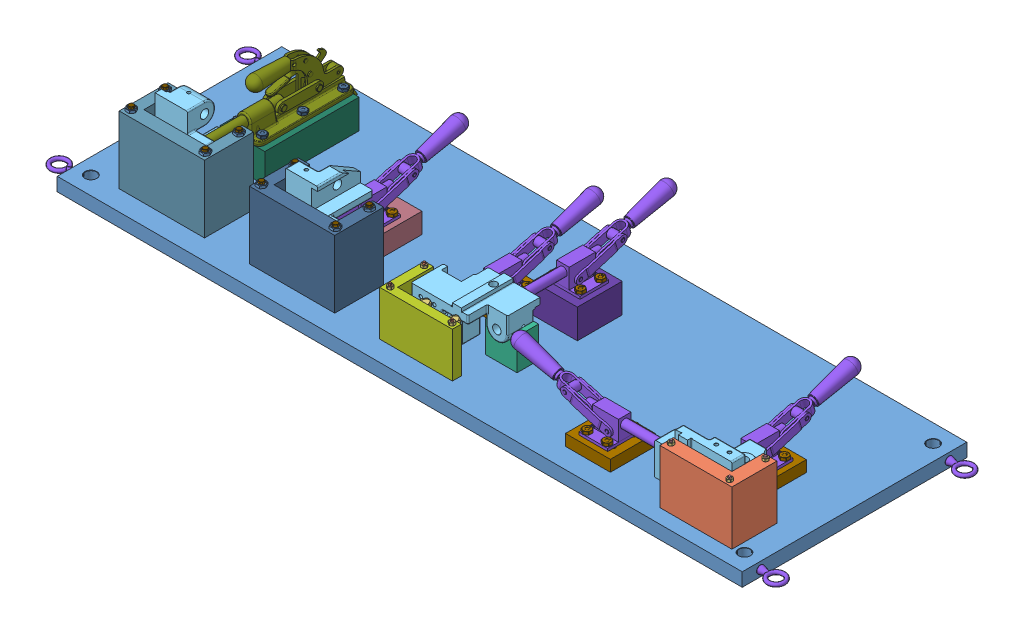
SolidWorks assembly Fixture Assy, configuration Default. Lengths in mm. (continued)
Mates (geometry in assembly coordinates): (continued)
- Coincident182: coincident anti-aligned: plane of Operation 1 Clamp Base-7 through (886.2945 606.2285 944.288) normal (0 1 0); plane of 5222N4_Heavy Duty Reverse-Action Push Toggle Clamp-7 through (854.2945 606.2285 982.288) normal (0 -1 0)
- Coincident183: coincident anti-aligned: plane of Roller Rest Bracket-1 through (1003.0152 704.2285 962.288) normal (-1 0 0); plane of 5222N4_Heavy Duty Reverse-Action Push Toggle Clamp-7 through (1003.0152 641.2285 944.288) normal (1 0 0)
- Distance93: distance = 45 mm aligned: plane of Operation 1 Clamp Base-7 through (836.2945 606.2285 994.288) normal (0 0 1); plane of Base-1 through (-724.9848 581.2285 1039.288) normal (0 0 1)
- Distance94: distance = 45 mm aligned: plane of Opeartion 3 BLock-1 through (322.5123 731.2285 994.288) normal (0 0 1); plane of Base-1 through (-724.9848 581.2285 1039.288) normal (0 0 1)
- Distance95: distance = 88 mm aligned: plane of U - BLock-Operation 2-1 through (422.5123 581.2285 994.288) normal (0 0 1); plane of Vee Block-1 through (570.5123 651.2285 906.288) normal (0 0 1)
- Coincident194: coincident aligned: plane of U - BLock-Operation 2-1 through (422.5123 581.2285 994.288) normal (0 0 1); plane of Opeartion 3 BLock-1 through (322.5123 731.2285 994.288) normal (0 0 1)
- Distance97: distance = 72 mm: cylinder of 2336A124_Locating Pin-18 through (424.5123 662.9738 902.288) axis (-1 0 0) radius 6; plane of U - BLock-Operation 2-1 through (644.5123 581.2285 974.288) normal (0 0 -1)
- Distance98: distance = 10 mm aligned: plane of 2336A124_Locating Pin-18 through (457.5123 671.2285 907.9324) normal (0 1 0); plane of U - BLock-Operation 2-1 through (543.5123 681.2285 974.288) normal (0 1 0)
- Width17: width anti-aligned: plane of Operation 2 Clamp Base-8 through (646.0152 646.2285 677.5673) normal (1 0 0); plane of 5222N4_Heavy Duty Reverse-Action Push Toggle Clamp-8 through (546.0152 646.2285 677.5673) normal (-1 0 0); plane of Operation 2 Clamp Base-8 through (558.0152 652.2285 759.5673) normal (-1 0 0); plane of 5222N4_Heavy Duty Reverse-Action Push Toggle Clamp-8 through (634.0152 652.2285 759.5673) normal (1 0 0)
- Width18: width anti-aligned: plane of Operation 2 Clamp Base-8 through (546.0152 646.2285 677.5673) normal (0 0 -1); plane of 5222N4_Heavy Duty Reverse-Action Push Toggle Clamp-8 through (546.0152 646.2285 777.5673) normal (0 0 1); plane of Operation 2 Clamp Base-8 through (634.0152 652.2285 759.5673) normal (0 0 1); plane of 5222N4_Heavy Duty Reverse-Action Push Toggle Clamp-8 through (634.0152 652.2285 695.5673) normal (0 0 -1)
- Coincident188: coincident anti-aligned: plane of 5222N4_Heavy Duty Reverse-Action Push Toggle Clamp-8 through (558.0152 646.2285 695.5673) normal (0 -1 0); plane of Operation 2 Clamp Base-8 through (596.0152 646.2285 727.5673) normal (0 1 0)
- Coincident193: coincident anti-aligned: plane of Base-1 through (275.0152 581.2285 789.288) normal (0 1 0); plane of Operation 2 Clamp Base-8 through (596.0152 581.2285 727.5673) normal (0 -1 0)
- Coincident195: coincident anti-aligned: plane of Roller Rest Bracket-2 through (457.5123 690.2285 844.288) normal (0 0 -1); plane of 5222N4_Heavy Duty Reverse-Action Push Toggle Clamp-8 through (596.0152 681.2285 844.288) normal (0 0 1)
- Distance100: distance = 6 mm anti-aligned: plane of Operation 1 Clamp Base-4 through (540.0152 606.2285 734.5673) normal (1 0 0); plane of Operation 2 Clamp Base-8 through (546.0152 646.2285 677.5673) normal (-1 0 0)
- Coincident198: coincident anti-aligned: plane of Base-1 through (275.0152 551.2285 789.288) normal (0 -1 0); plane of 93516A178_Bronze Hex Head Screw-2 through (321.0108 551.2285 904.813) normal (0 1 0)
- Coincident199: coincident anti-aligned: plane of Base-1 through (275.0152 551.2285 789.288) normal (0 -1 0); plane of 93516A178_Bronze Hex Head Screw-2 through (321.0108 551.2285 904.813) normal (0 1 0)
- Coincident200: coincident anti-aligned: plane of Base-1 through (275.0152 551.2285 789.288) normal (0 -1 0); plane of 93516A178_Bronze Hex Head Screw-3 through (-139.4885 551.2285 989.288) normal (0 1 0)
- Coincident201: coincident anti-aligned: plane of Base-1 through (275.0152 551.2285 789.288) normal (0 -1 0); plane of 93516A178_Bronze Hex Head Screw-4 through (150.5115 551.2285 914.338) normal (0 1 0)
- Coincident202: coincident anti-aligned: plane of Base-1 through (275.0152 551.2285 789.288) normal (0 -1 0); plane of 93516A178_Bronze Hex Head Screw-5 through (315.5115 551.2285 989.288) normal (0 1 0)
- Coincident203: coincident anti-aligned: plane of Base-1 through (275.0152 551.2285 789.288) normal (0 -1 0); plane of 93516A178_Bronze Hex Head Screw-8 through (31.0108 551.2285 904.813) normal (0 1 0)
- Coincident204: coincident anti-aligned: plane of Base-1 through (275.0152 551.2285 789.288) normal (0 -1 0); plane of 93516A178_Bronze Hex Head Screw-9 through (-133.9892 551.2285 904.813) normal (0 1 0)
- Coincident205: coincident anti-aligned: plane of Base-1 through (275.0152 551.2285 789.288) normal (0 -1 0); plane of 93516A178_Bronze Hex Head Screw-7 through (150.5115 551.2285 989.288) normal (0 1 0)
- Coincident206: coincident anti-aligned: plane of Base-1 through (275.0152 551.2285 789.288) normal (0 -1 0); plane of 93516A178_Bronze Hex Head Screw-6 through (31.0108 551.2285 979.763) normal (0 1 0)
- Distance101: distance = 10 mm aligned: plane of Opeartion 3 BLock-1 through (297.5123 731.2285 885.288) normal (0 0 -1); plane of 93516A178_Bronze Hex Head Screw-2 through (304.513 543.291 895.288) normal (0 0 -1)
- Width19: width: plane of Opeartion 3 BLock-1 through (322.5123 731.2285 885.288) normal (1 0 0); plane of Opeartion 3 BLock-1 through (297.5123 731.2285 964.288) normal (-1 0 0); cylinder of 93516A178_Bronze Hex Head Screw-2 through (310.0123 741.7285 904.813) axis (0 1 0) radius 6.35
- Width20: width: plane of Opeartion 3 BLock-1 through (132.5123 731.2285 994.288) normal (-1 0 0); plane of Opeartion 3 BLock-1 through (157.5123 731.2285 885.288) normal (1 0 0); cylinder of 93516A178_Bronze Hex Head Screw-4 through (145.0123 741.7285 904.813) axis (0 1 0) radius 6.35
- Width21: width: plane of Opeartion 3 BLock-1 through (157.5123 731.2285 885.288) normal (1 0 0); plane of Opeartion 3 BLock-1 through (132.5123 731.2285 994.288) normal (-1 0 0); cylinder of 93516A178_Bronze Hex Head Screw-7 through (145.0123 741.7285 979.763) axis (0 1 0) radius 6.35
- Width22: width: plane of Opeartion 3 BLock-1 through (297.5123 731.2285 964.288) normal (-1 0 0); plane of Opeartion 3 BLock-1 through (322.5123 731.2285 885.288) normal (1 0 0); cylinder of 93516A178_Bronze Hex Head Screw-5 through (310.0123 741.7285 979.763) axis (0 1 0) radius 6.35
- Width23: width: plane of Opeartion 4 BLock-2 through (32.5123 731.2285 885.288) normal (1 0 0); plane of Opeartion 4 BLock-2 through (7.5123 731.2285 964.288) normal (-1 0 0); cylinder of 93516A178_Bronze Hex Head Screw-8 through (20.0123 741.7285 904.813) axis (0 1 0) radius 6.35
- Width24: width: plane of Opeartion 4 BLock-2 through (7.5123 731.2285 964.288) normal (-1 0 0); plane of Opeartion 4 BLock-2 through (32.5123 731.2285 885.288) normal (1 0 0); cylinder of 93516A178_Bronze Hex Head Screw-6 through (20.0123 741.7285 979.763) axis (0 1 0) radius 6.35
- Width25: width: plane of Opeartion 4 BLock-2 through (-132.4877 731.2285 885.288) normal (1 0 0); plane of Opeartion 4 BLock-2 through (-157.4877 731.2285 994.288) normal (-1 0 0); cylinder of 93516A178_Bronze Hex Head Screw-9 through (-144.9877 741.7285 904.813) axis (0 1 0) radius 6.35
- Width26: width: plane of Opeartion 4 BLock-2 through (-157.4877 731.2285 994.288) normal (-1 0 0); plane of Opeartion 4 BLock-2 through (-132.4877 731.2285 885.288) normal (1 0 0); cylinder of 93516A178_Bronze Hex Head Screw-3 through (-144.9877 741.7285 979.763) axis (0 1 0) radius 6.35
- Coincident210: coincident aligned: plane of 93516A178_Bronze Hex Head Screw-2 through (304.513 543.291 895.288) normal (0 0 -1); plane of 93516A178_Bronze Hex Head Screw-4 through (139.513 543.291 895.288) normal (0 0 -1)
- Coincident211: coincident aligned: plane of 93516A178_Bronze Hex Head Screw-2 through (304.513 543.291 895.288) normal (0 0 -1); plane of 93516A178_Bronze Hex Head Screw-8 through (14.513 543.291 895.288) normal (0 0 -1)
- Coincident212: coincident aligned: plane of 93516A178_Bronze Hex Head Screw-8 through (14.513 543.291 895.288) normal (0 0 -1); plane of 93516A178_Bronze Hex Head Screw-9 through (-150.487 543.291 895.288) normal (0 0 -1)
- Distance102: distance = 5 mm aligned: plane of 93516A178_Bronze Hex Head Screw-5 through (315.5115 543.291 989.288) normal (0 0 1); plane of Opeartion 3 BLock-1 through (322.5123 731.2285 994.288) normal (0 0 1)
- Coincident214: coincident aligned: plane of 93516A178_Bronze Hex Head Screw-5 through (315.5115 543.291 989.288) normal (0 0 1); plane of 93516A178_Bronze Hex Head Screw-7 through (150.5115 543.291 989.288) normal (0 0 1)
- Coincident215: coincident aligned: plane of 93516A178_Bronze Hex Head Screw-6 through (25.5115 543.291 989.288) normal (0 0 1); plane of 93516A178_Bronze Hex Head Screw-7 through (150.5115 543.291 989.288) normal (0 0 1)
- Coincident216: coincident aligned: plane of 93516A178_Bronze Hex Head Screw-3 through (-139.4885 543.291 989.288) normal (0 0 1); plane of 93516A178_Bronze Hex Head Screw-6 through (25.5115 543.291 989.288) normal (0 0 1)
- Coincident220: coincident anti-aligned: plane of Opeartion 3 BLock-1 through (227.5123 731.2285 994.288) normal (0 1 0); plane of 98886A736_High-Strength High-Temperature PEEK Hex Nut-2 through (310.0123 731.2285 904.813) normal (0 -1 0)
- Concentric3: concentric aligned: circle of 93516A178_Bronze Hex Head Screw-2; circle of 98886A736_High-Strength High-Temperature PEEK Hex Nut-2
- Coincident221: coincident anti-aligned: plane of Opeartion 3 BLock-1 through (227.5123 731.2285 994.288) normal (0 1 0); plane of 98886A736_High-Strength High-Temperature PEEK Hex Nut-3 through (310.0123 731.2285 979.763) normal (0 -1 0)
- Concentric4: concentric anti-aligned: circle of 93516A178_Bronze Hex Head Screw-5; circle of 98886A736_High-Strength High-Temperature PEEK Hex Nut-3
- Concentric5: concentric anti-aligned: circle of 93516A178_Bronze Hex Head Screw-7; circle of 98886A736_High-Strength High-Temperature PEEK Hex Nut-4
- Coincident222: coincident anti-aligned: plane of Opeartion 3 BLock-1 through (227.5123 731.2285 994.288) normal (0 1 0); plane of 98886A736_High-Strength High-Temperature PEEK Hex Nut-4 through (145.0123 731.2285 979.763) normal (0 -1 0)
- Coincident223: coincident anti-aligned: plane of Opeartion 3 BLock-1 through (227.5123 731.2285 994.288) normal (0 1 0); plane of 98886A736_High-Strength High-Temperature PEEK Hex Nut-5 through (145.0123 731.2285 904.813) normal (0 -1 0)
- Concentric6: concentric anti-aligned: circle of 93516A178_Bronze Hex Head Screw-4; circle of 98886A736_High-Strength High-Temperature PEEK Hex Nut-5
- Coincident224: coincident anti-aligned: plane of Opeartion 4 BLock-2 through (-62.4877 731.2285 994.288) normal (0 1 0); plane of 98886A736_High-Strength High-Temperature PEEK Hex Nut-9 through (20.0123 731.2285 904.813) normal (0 -1 0)
- Concentric7: concentric anti-aligned: circle of 93516A178_Bronze Hex Head Screw-8; circle of 98886A736_High-Strength High-Temperature PEEK Hex Nut-9
- Coincident225: coincident anti-aligned: plane of Opeartion 4 BLock-2 through (-62.4877 731.2285 994.288) normal (0 1 0); plane of 98886A736_High-Strength High-Temperature PEEK Hex Nut-8 through (20.0123 731.2285 979.763) normal (0 -1 0)
- Concentric8: concentric anti-aligned: circle of 93516A178_Bronze Hex Head Screw-6; circle of 98886A736_High-Strength High-Temperature PEEK Hex Nut-8
- Coincident226: coincident anti-aligned: plane of Opeartion 4 BLock-2 through (-62.4877 731.2285 994.288) normal (0 1 0); plane of 98886A736_High-Strength High-Temperature PEEK Hex Nut-6 through (-144.9877 731.2285 979.763) normal (0 -1 0)
- Concentric9: concentric anti-aligned: circle of 93516A178_Bronze Hex Head Screw-3; circle of 98886A736_High-Strength High-Temperature PEEK Hex Nut-6
- Coincident227: coincident anti-aligned: plane of Opeartion 4 BLock-2 through (-62.4877 731.2285 994.288) normal (0 1 0); plane of 98886A736_High-Strength High-Temperature PEEK Hex Nut-7 through (-144.9877 731.2285 904.813) normal (0 -1 0)
- Concentric10: concentric anti-aligned: circle of 93516A178_Bronze Hex Head Screw-9; circle of 98886A736_High-Strength High-Temperature PEEK Hex Nut-7
- Coincident229: coincident anti-aligned: plane of Base-1 through (275.0152 551.2285 789.288) normal (0 -1 0); plane of 91268A514_High-Strength Grade 8 Steel Hex Head Screw-1 through (435.7202 551.2285 899.288) normal (0 1 0)
- Coincident230: coincident anti-aligned: plane of Base-1 through (275.0152 551.2285 789.288) normal (0 -1 0); plane of 91268A514_High-Strength Grade 8 Steel Hex Head Screw-2 through (438.7694 551.2285 989.288) normal (0 1 0)
- Coincident231: coincident anti-aligned: plane of Base-1 through (275.0152 551.2285 789.288) normal (0 -1 0); plane of 91268A514_High-Strength Grade 8 Steel Hex Head Screw-3 through (573.956 551.2285 990.7038) normal (0 1 0)
- Distance103: distance = 5 mm aligned: plane of 91268A514_High-Strength Grade 8 Steel Hex Head Screw-2 through (438.7694 547.2598 989.288) normal (0 0 1); plane of U - BLock-Operation 2-1 through (422.5123 581.2285 994.288) normal (0 0 1)
- Distance104: distance = 5 mm aligned: plane of 91268A514_High-Strength Grade 8 Steel Hex Head Screw-1 through (429.3044 547.2598 899.288) normal (0 0 -1); plane of U - BLock-Operation 2-1 through (442.5123 581.2285 894.288) normal (0 0 -1)
- Distance105: distance = 5 mm aligned: plane of 91268A514_High-Strength Grade 8 Steel Hex Head Screw-3 through (579.5123 547.2598 981.0801) normal (1 0 0); plane of U - BLock-Operation 2-1 through (584.5123 581.2285 894.288) normal (1 0 0)
- Width32: width: plane of U - BLock-Operation 2-1 through (422.5123 581.2285 994.288) normal (0 0 1); plane of U - BLock-Operation 2-1 through (644.5123 581.2285 974.288) normal (0 0 -1); cylinder of 91268A514_High-Strength Grade 8 Steel Hex Head Screw-3 through (573.956 538.5335 984.288) axis (0 1 0) radius 3.175
- Width34: width: plane of U - BLock-Operation 2-1 through (422.5123 581.2285 894.288) normal (-1 0 0); plane of U - BLock-Operation 2-1 through (442.5123 581.2285 974.288) normal (1 0 0); cylinder of 91268A514_High-Strength Grade 8 Steel Hex Head Screw-1 through (432.5123 538.5335 904.8443) axis (0 1 0) radius 3.175
- Coincident243: coincident anti-aligned: plane of U - BLock-Operation 2-1 through (543.5123 681.2285 974.288) normal (0 1 0); plane of 95462A029_Medium-Strength Steel Hex Nut-1 through (435.5615 681.2285 983.7318) normal (0 -1 0)
- Concentric11: concentric anti-aligned: circle of 91268A514_High-Strength Grade 8 Steel Hex Head Screw-2; circle of 95462A029_Medium-Strength Steel Hex Nut-1
- Coincident244: coincident anti-aligned: plane of U - BLock-Operation 2-1 through (543.5123 681.2285 974.288) normal (0 1 0); plane of 95462A029_Medium-Strength Steel Hex Nut-2 through (432.5123 681.2285 904.8443) normal (0 -1 0)
- Concentric12: concentric aligned: circle of 91268A514_High-Strength Grade 8 Steel Hex Head Screw-1; circle of 95462A029_Medium-Strength Steel Hex Nut-2
- Coincident245: coincident anti-aligned: plane of U - BLock-Operation 2-1 through (543.5123 681.2285 974.288) normal (0 1 0); plane of 95462A029_Medium-Strength Steel Hex Nut-4 through (573.956 681.2285 984.288) normal (0 -1 0)
- Concentric13: concentric anti-aligned: circle of 91268A514_High-Strength Grade 8 Steel Hex Head Screw-3; circle of 95462A029_Medium-Strength Steel Hex Nut-4
- Coincident248: coincident anti-aligned: plane of Base-1 through (275.0152 551.2285 789.288) normal (0 -1 0); plane of 91251A562_Black-Oxide Alloy Steel Socket Head Screw-1 through (1204.5795 551.2285 1000.433) normal (0 1 0)
- Coincident249: coincident anti-aligned: plane of Base-1 through (275.0152 551.2285 789.288) normal (0 -1 0); plane of 91251A562_Black-Oxide Alloy Steel Socket Head Screw-3 through (1069.5123 551.2285 995.463) normal (0 1 0)
- Coincident250: coincident anti-aligned: plane of Base-1 through (275.0152 551.2285 789.288) normal (0 -1 0); plane of 91251A562_Black-Oxide Alloy Steel Socket Head Screw-2 through (1205.0152 551.2285 920.463) normal (0 1 0)
- Width35: width: plane of U_Block-1 through (1220.0152 701.2285 907.288) normal (1 0 0); plane of U_Block-1 through (1190.0152 701.2285 977.288) normal (-1 0 0); cylinder of 91251A562_Black-Oxide Alloy Steel Socket Head Screw-2 through (1205.0152 542.1046 917.288) axis (0 1 0) radius 3.2258
- Width36: width: plane of U_Block-1 through (1190.0152 701.2285 977.288) normal (-1 0 0); plane of U_Block-1 through (1220.0152 701.2285 907.288) normal (1 0 0); cylinder of 91251A562_Black-Oxide Alloy Steel Socket Head Screw-1 through (1205.0152 542.1046 997.288) axis (0 1 0) radius 3.2258
- Width37: width: plane of U_Block-1 through (991.0152 701.2285 977.288) normal (0 0 -1); plane of U_Block-1 through (1220.0152 701.2285 1007.288) normal (0 0 1); cylinder of 91251A562_Black-Oxide Alloy Steel Socket Head Screw-3 through (1069.5123 542.1046 992.288) axis (0 1 0) radius 3.2258
- Distance109: distance = 10 mm: cylinder of 91251A562_Black-Oxide Alloy Steel Socket Head Screw-3 through (1069.5123 542.1046 992.288) axis (0 1 0) radius 3.2258; plane of U_Block-1 through (1059.5123 701.2285 1007.288) normal (-1 0 0)
- Distance110: distance = 10 mm: cylinder of 91251A562_Black-Oxide Alloy Steel Socket Head Screw-1 through (1205.0152 542.1046 997.288) axis (0 1 0) radius 3.2258; plane of U_Block-1 through (1220.0152 701.2285 1007.288) normal (0 0 1)
- Distance111: distance = 10 mm: cylinder of 91251A562_Black-Oxide Alloy Steel Socket Head Screw-2 through (1205.0152 542.1046 917.288) axis (0 1 0) radius 3.2258; plane of U_Block-1 through (1190.0152 701.2285 907.288) normal (0 0 -1)
- Coincident251: coincident anti-aligned: plane of U_Block-1 through (1090.5152 701.2285 977.288) normal (0 1 0); plane of 95462A029_Medium-Strength Steel Hex Nut-5 through (1069.5123 701.2285 992.288) normal (0 -1 0)
- Concentric14: concentric aligned: circle of 91251A562_Black-Oxide Alloy Steel Socket Head Screw-3; circle of 95462A029_Medium-Strength Steel Hex Nut-5
- Coincident252: coincident anti-aligned: plane of U_Block-1 through (1090.5152 701.2285 977.288) normal (0 1 0); plane of 95462A029_Medium-Strength Steel Hex Nut-6 through (1205.0152 701.2285 997.288) normal (0 -1 0)
- Concentric15: concentric anti-aligned: circle of 91251A562_Black-Oxide Alloy Steel Socket Head Screw-1; circle of 95462A029_Medium-Strength Steel Hex Nut-6
- Coincident253: coincident anti-aligned: plane of U_Block-1 through (1090.5152 701.2285 977.288) normal (0 1 0); plane of 95462A029_Medium-Strength Steel Hex Nut-7 through (1205.0152 701.2285 917.288) normal (0 -1 0)
- Concentric16: concentric anti-aligned: circle of 91251A562_Black-Oxide Alloy Steel Socket Head Screw-2; circle of 95462A029_Medium-Strength Steel Hex Nut-7
- Coincident2551: coincident anti-aligned: plane of Base-1 through (275.0152 551.2285 789.288) normal (0 -1 0); plane of 91257A550_Zinc Yellow-Chromate Plated Hex Head Screw (1)-1 through (631.3915 551.2285 693.6798) normal (0 1 0)
- Coincident2561: coincident anti-aligned: plane of Base-1 through (275.0152 551.2285 789.288) normal (0 -1 0); plane of 91257A550_Zinc Yellow-Chromate Plated Hex Head Screw (1)-2 through (554.2231 551.2285 693.6798) normal (0 1 0)
- Coincident2571: coincident anti-aligned: plane of Base-1 through (275.0152 551.2285 789.288) normal (0 -1 0); plane of 91257A550_Zinc Yellow-Chromate Plated Hex Head Screw (1)-3 through (554.2231 551.2285 772.5673) normal (0 1 0)
- Coincident2581: coincident anti-aligned: plane of Base-1 through (275.0152 551.2285 789.288) normal (0 -1 0); plane of 91257A550_Zinc Yellow-Chromate Plated Hex Head Screw (1)-4 through (631.3915 551.2285 772.5673) normal (0 1 0)
- Distance112: distance = 5 mm aligned: plane of Operation 2 Clamp Base-8 through (546.0152 646.2285 677.5673) normal (0 0 -1); plane of 91257A550_Zinc Yellow-Chromate Plated Hex Head Screw (1)-1 through (631.3915 546.8629 682.5673) normal (0 0 -1)
- Distance113: distance = 5 mm aligned: plane of 91257A550_Zinc Yellow-Chromate Plated Hex Head Screw (1)-4 through (637.8073 546.8629 772.5673) normal (0 0 1); plane of Operation 2 Clamp Base-8 through (546.0152 646.2285 777.5673) normal (0 0 1)
- Distance114: distance = 5 mm aligned: plane of 91257A550_Zinc Yellow-Chromate Plated Hex Head Screw (1)-3 through (560.6389 546.8629 772.5673) normal (0 0 1); plane of Operation 2 Clamp Base-8 through (546.0152 646.2285 777.5673) normal (0 0 1)
- Distance115: distance = 5 mm aligned: plane of Operation 2 Clamp Base-8 through (546.0152 646.2285 677.5673) normal (0 0 -1); plane of 91257A550_Zinc Yellow-Chromate Plated Hex Head Screw (1)-2 through (554.2231 546.8629 682.5673) normal (0 0 -1)
- Distance116: distance = 5 mm: line of 91257A550_Zinc Yellow-Chromate Plated Hex Head Screw (1)-1 through (641.0152 547.3592 688.1236) axis (0 1 0); plane of Operation 2 Clamp Base-8 through (646.0152 646.2285 677.5673) normal (1 0 0)
- Parallel4: parallel aligned: line of 91257A550_Zinc Yellow-Chromate Plated Hex Head Screw (1)-1 through (641.0152 547.3592 688.1236) axis (0 1 0); line of 91257A550_Zinc Yellow-Chromate Plated Hex Head Screw (1)-4 through (641.0152 547.3592 767.0111) axis (0 1 0)
- Distance117: distance = 5 mm: point of 91257A550_Zinc Yellow-Chromate Plated Hex Head Screw (1)-2; plane of Operation 2 Clamp Base-8 through (546.0152 646.2285 677.5673) normal (-1 0 0)
- Distance118: distance = 5 mm: line of 91257A550_Zinc Yellow-Chromate Plated Hex Head Screw (1)-3 through (551.0152 547.3592 767.0111) axis (0 1 0); plane of Operation 2 Clamp Base-8 through (546.0152 646.2285 677.5673) normal (-1 0 0)
- Coincident2583: coincident anti-aligned: plane of Base-1 through (275.0152 551.2285 789.288) normal (0 -1 0); plane of 91257A550_Zinc Yellow-Chromate Plated Hex Head Screw (1)-8 through (-10.1927 551.2285 631.6331) normal (0 1 0)
- Coincident2584: coincident anti-aligned: plane of Base-1 through (275.0152 551.2285 789.288) normal (0 -1 0); plane of 91257A550_Zinc Yellow-Chromate Plated Hex Head Screw (1)-6 through (-16.6085 551.2285 820.5206) normal (0 1 0)
- Coincident2585: coincident anti-aligned: plane of Base-1 through (275.0152 551.2285 789.288) normal (0 -1 0); plane of 91257A550_Zinc Yellow-Chromate Plated Hex Head Screw (1)-5 through (-87.3611 551.2285 820.5206) normal (0 1 0)
- Coincident2586: coincident anti-aligned: plane of Base-1 through (275.0152 551.2285 789.288) normal (0 -1 0); plane of 91257A550_Zinc Yellow-Chromate Plated Hex Head Screw (1)-7 through (-93.7769 551.2285 631.6331) normal (0 1 0)
- Distance119: distance = 5 mm aligned: plane of 91257A550_Zinc Yellow-Chromate Plated Hex Head Screw (1)-8 through (-16.6085 546.8629 620.5206) normal (0 0 -1); plane of Op 4 Clamp base-6 through (-101.9848 646.2285 615.5206) normal (0 0 -1)
- Distance120: distance = 5 mm: line of 91257A550_Zinc Yellow-Chromate Plated Hex Head Screw (1)-8 through (-6.9848 547.3592 626.0769) axis (0 1 0); plane of Op 4 Clamp base-6 through (-1.9848 646.2285 615.5206) normal (1 0 0)
- Coincident2589: coincident aligned: plane of 91257A550_Zinc Yellow-Chromate Plated Hex Head Screw (1)-7 through (-93.7769 546.8629 620.5206) normal (0 0 -1); plane of 91257A550_Zinc Yellow-Chromate Plated Hex Head Screw (1)-8 through (-16.6085 546.8629 620.5206) normal (0 0 -1)
- Distance121: distance = 5 mm: line of 91257A550_Zinc Yellow-Chromate Plated Hex Head Screw (1)-7 through (-96.9848 547.3592 626.0769) axis (0 1 0); plane of Op 4 Clamp base-6 through (-101.9848 646.2285 615.5206) normal (-1 0 0)
- Distance122: distance = 5 mm aligned: plane of 91257A550_Zinc Yellow-Chromate Plated Hex Head Screw (1)-6 through (-10.1927 546.8629 820.5206) normal (0 0 1); plane of Op 4 Clamp base-6 through (-101.9848 646.2285 825.5206) normal (0 0 1)
- Distance123: distance = 5 mm aligned: plane of 91257A550_Zinc Yellow-Chromate Plated Hex Head Screw (1)-5 through (-87.3611 546.8629 820.5206) normal (0 0 1); plane of Op 4 Clamp base-6 through (-101.9848 646.2285 825.5206) normal (0 0 1)
- Distance124: distance = 5 mm: line of 91257A550_Zinc Yellow-Chromate Plated Hex Head Screw (1)-6 through (-6.9848 547.3592 814.9644) axis (0 1 0); plane of Op 4 Clamp base-6 through (-1.9848 646.2285 615.5206) normal (1 0 0)
- Distance125: distance = 5 mm: plane of Op 4 Clamp base-6 through (-101.9848 646.2285 615.5206) normal (-1 0 0); line of 91257A550_Zinc Yellow-Chromate Plated Hex Head Screw (1)-5 through (-96.9848 547.3592 814.9644) axis (0 1 0)
- Coincident2595: coincident anti-aligned: plane of Base-1 through (275.0152 551.2285 789.288) normal (0 -1 0); plane of 91257A552_Zinc Yellow-Chromate Plated Hex Head Screw-2 through (253.3915 551.2285 761.6798) normal (0 1 0)
- Coincident2607: coincident anti-aligned: plane of Base-1 through (275.0152 551.2285 789.288) normal (0 -1 0); plane of 91257A552_Zinc Yellow-Chromate Plated Hex Head Screw-4 through (176.2231 551.2285 761.6798) normal (0 1 0)
- Coincident2597: coincident anti-aligned: plane of Base-1 through (275.0152 551.2285 789.288) normal (0 -1 0); plane of 91257A552_Zinc Yellow-Chromate Plated Hex Head Screw-3 through (253.3915 551.2285 840.5673) normal (0 1 0)
- Coincident2598: coincident anti-aligned: plane of Base-1 through (275.0152 551.2285 789.288) normal (0 -1 0); plane of 91257A552_Zinc Yellow-Chromate Plated Hex Head Screw-1 through (176.2231 551.2285 840.5673) normal (0 1 0)
- Distance126: distance = 5 mm aligned: plane of Operation 3 Clamp Base-5 through (168.0152 626.2285 745.5673) normal (0 0 -1); plane of 91257A552_Zinc Yellow-Chromate Plated Hex Head Screw-2 through (253.3915 546.8629 750.5673) normal (0 0 -1)
- Distance127: distance = 5 mm aligned: plane of 91257A552_Zinc Yellow-Chromate Plated Hex Head Screw-4 through (176.2231 546.8629 750.5673) normal (0 0 -1); plane of Operation 3 Clamp Base-5 through (168.0152 626.2285 745.5673) normal (0 0 -1)
- Distance128: distance = 5 mm aligned: plane of 91257A552_Zinc Yellow-Chromate Plated Hex Head Screw-3 through (259.8073 546.8629 840.5673) normal (0 0 1); plane of Operation 3 Clamp Base-5 through (168.0152 626.2285 845.5673) normal (0 0 1)
- Distance129: distance = 5 mm aligned: plane of 91257A552_Zinc Yellow-Chromate Plated Hex Head Screw-1 through (182.6389 546.8629 840.5673) normal (0 0 1); plane of Operation 3 Clamp Base-5 through (168.0152 626.2285 845.5673) normal (0 0 1)
- Distance130: distance = 5 mm: plane of 91257A552_Zinc Yellow-Chromate Plated Hex Head Screw-2; plane of Operation 3 Clamp Base-5 through (268.0152 626.2285 745.5673) normal (1 0 0)
- Distance131: distance = 5 mm: plane of Operation 3 Clamp Base-5 through (268.0152 626.2285 745.5673) normal (1 0 0); line of 91257A552_Zinc Yellow-Chromate Plated Hex Head Screw-3 through (263.0152 547.3592 835.0111) axis (0 1 0)
- Distance132: distance = 5 mm: plane of Operation 3 Clamp Base-5 through (168.0152 626.2285 745.5673) normal (-1 0 0); line of 91257A552_Zinc Yellow-Chromate Plated Hex Head Screw-4 through (173.0152 547.3592 756.1236) axis (0 1 0)
- Distance133: distance = 5 mm: plane of Operation 3 Clamp Base-5 through (168.0152 626.2285 745.5673) normal (-1 0 0); line of 91257A552_Zinc Yellow-Chromate Plated Hex Head Screw-1 through (173.0152 547.3592 835.0111) axis (0 1 0)
- Coincident2608: coincident anti-aligned: plane of Base-1 through (275.0152 551.2285 789.288) normal (0 -1 0); plane of 91257A546_Zinc Yellow-Chromate Plated Hex Head Screw-1 through (525.3915 551.2285 750.6798) normal (0 1 0)
- Coincident2609: coincident anti-aligned: plane of Base-1 through (275.0152 551.2285 789.288) normal (0 -1 0); plane of 91257A546_Zinc Yellow-Chromate Plated Hex Head Screw-4 through (448.2231 551.2285 750.6798) normal (0 1 0)
- Coincident2610: coincident anti-aligned: plane of Base-1 through (275.0152 551.2285 789.288) normal (0 -1 0); plane of 91257A546_Zinc Yellow-Chromate Plated Hex Head Screw-3 through (525.3915 551.2285 829.5673) normal (0 1 0)
- Coincident2611: coincident anti-aligned: plane of Base-1 through (275.0152 551.2285 789.288) normal (0 -1 0); plane of 91257A546_Zinc Yellow-Chromate Plated Hex Head Screw-2 through (448.2231 551.2285 829.5673) normal (0 1 0)
- Coincident2612: coincident anti-aligned: plane of Base-1 through (275.0152 551.2285 789.288) normal (0 -1 0); plane of 91257A546_Zinc Yellow-Chromate Plated Hex Head Screw-5 through (844.5024 551.2285 989.288) normal (0 1 0)
- Coincident2613: coincident anti-aligned: plane of Base-1 through (275.0152 551.2285 789.288) normal (0 -1 0); plane of 91257A546_Zinc Yellow-Chromate Plated Hex Head Screw-6 through (844.5024 551.2285 910.4005) normal (0 1 0)
- Coincident2614: coincident anti-aligned: plane of Base-1 through (275.0152 551.2285 789.288) normal (0 -1 0); plane of 91257A546_Zinc Yellow-Chromate Plated Hex Head Screw-7 through (921.6708 551.2285 910.4005) normal (0 1 0)
- Coincident2615: coincident anti-aligned: plane of Base-1 through (275.0152 551.2285 789.288) normal (0 -1 0); plane of 91257A546_Zinc Yellow-Chromate Plated Hex Head Screw-8 through (921.6708 551.2285 989.288) normal (0 1 0)
- Distance135: distance = 5 mm aligned: plane of Operation 1 Clamp Base-4 through (440.0152 606.2285 734.5673) normal (0 0 -1); plane of 91257A546_Zinc Yellow-Chromate Plated Hex Head Screw-4 through (448.2231 546.8629 739.5673) normal (0 0 -1)
- Distance136: distance = 5 mm aligned: plane of Operation 1 Clamp Base-4 through (440.0152 606.2285 734.5673) normal (0 0 -1); plane of 91257A546_Zinc Yellow-Chromate Plated Hex Head Screw-1 through (525.3915 546.8629 739.5673) normal (0 0 -1)
- Distance137: distance = 5 mm aligned: plane of Operation 1 Clamp Base-4 through (440.0152 606.2285 834.5673) normal (0 0 1); plane of 91257A546_Zinc Yellow-Chromate Plated Hex Head Screw-3 through (531.8073 546.8629 829.5673) normal (0 0 1)
- Distance138: distance = 5 mm aligned: plane of Operation 1 Clamp Base-4 through (440.0152 606.2285 834.5673) normal (0 0 1); plane of 91257A546_Zinc Yellow-Chromate Plated Hex Head Screw-2 through (454.6389 546.8629 829.5673) normal (0 0 1)
- Distance139: distance = 5 mm: line of 91257A546_Zinc Yellow-Chromate Plated Hex Head Screw-3 through (535.0152 547.3592 824.0111) axis (0 1 0); plane of Operation 1 Clamp Base-4 through (540.0152 606.2285 734.5673) normal (1 0 0)
- Distance140: distance = 5 mm: plane of Operation 1 Clamp Base-4 through (440.0152 606.2285 734.5673) normal (-1 0 0); line of 91257A546_Zinc Yellow-Chromate Plated Hex Head Screw-2 through (445.0152 547.3592 824.0111) axis (0 1 0)
- Distance141: distance = 5 mm: plane of Operation 1 Clamp Base-4 through (440.0152 606.2285 734.5673) normal (-1 0 0); line of 91257A546_Zinc Yellow-Chromate Plated Hex Head Screw-4 through (445.0152 547.3592 745.1236) axis (0 1 0)
- Distance142: distance = 5 mm: line of 91257A546_Zinc Yellow-Chromate Plated Hex Head Screw-1 through (535.0152 547.3592 745.1236) axis (0 1 0); plane of Operation 1 Clamp Base-4 through (540.0152 606.2285 734.5673) normal (1 0 0)
- Distance143: distance = 5 mm aligned: plane of Operation 1 Clamp Base-7 through (836.2945 606.2285 894.288) normal (0 0 -1); plane of 91257A546_Zinc Yellow-Chromate Plated Hex Head Screw-7 through (921.6708 546.8629 899.288) normal (0 0 -1)
- Distance144: distance = 5 mm aligned: plane of 91257A546_Zinc Yellow-Chromate Plated Hex Head Screw-6 through (844.5024 546.8629 899.288) normal (0 0 -1); plane of Operation 1 Clamp Base-7 through (836.2945 606.2285 894.288) normal (0 0 -1)
- Distance145: distance = 5 mm aligned: plane of 91257A546_Zinc Yellow-Chromate Plated Hex Head Screw-8 through (928.0866 546.8629 989.288) normal (0 0 1); plane of Operation 1 Clamp Base-7 through (836.2945 606.2285 994.288) normal (0 0 1)
- Distance146: distance = 5 mm aligned: plane of Operation 1 Clamp Base-7 through (836.2945 606.2285 994.288) normal (0 0 1); plane of 91257A546_Zinc Yellow-Chromate Plated Hex Head Screw-5 through (850.9182 546.8629 989.288) normal (0 0 1)
- Distance147: distance = 5 mm: plane of Operation 1 Clamp Base-7 through (836.2945 606.2285 894.288) normal (-1 0 0); line of 91257A546_Zinc Yellow-Chromate Plated Hex Head Screw-5 through (841.2945 547.3592 983.7318) axis (0 1 0)
- Distance148: distance = 5 mm: plane of Operation 1 Clamp Base-7 through (836.2945 606.2285 894.288) normal (-1 0 0); line of 91257A546_Zinc Yellow-Chromate Plated Hex Head Screw-6 through (841.2945 547.3592 904.8443) axis (0 1 0)
- Distance149: distance = 5 mm: plane of Operation 1 Clamp Base-7 through (936.2945 606.2285 894.288) normal (1 0 0); line of 91257A546_Zinc Yellow-Chromate Plated Hex Head Screw-7 through (931.2945 547.3592 904.8443) axis (0 1 0)
- Distance150: distance = 5 mm: plane of Operation 1 Clamp Base-7 through (936.2945 606.2285 894.288) normal (1 0 0); line of 91257A546_Zinc Yellow-Chromate Plated Hex Head Screw-8 through (931.2945 547.3592 983.7318) axis (0 1 0)
- Coincident2632: coincident anti-aligned: plane of Base-1 through (275.0152 551.2285 789.288) normal (0 -1 0); plane of 91257A546_Zinc Yellow-Chromate Plated Hex Head Screw-10 through (1140.3915 551.2285 871.5673) normal (0 1 0)
- Coincident2633: coincident anti-aligned: plane of Base-1 through (275.0152 551.2285 789.288) normal (0 -1 0); plane of 91257A546_Zinc Yellow-Chromate Plated Hex Head Screw-11 through (1063.2231 551.2285 871.5673) normal (0 1 0)
- Coincident2634: coincident anti-aligned: plane of Base-1 through (275.0152 551.2285 789.288) normal (0 -1 0); plane of 91257A546_Zinc Yellow-Chromate Plated Hex Head Screw-12 through (1063.2231 551.2285 792.6798) normal (0 1 0)
- Coincident2635: coincident anti-aligned: plane of Base-1 through (275.0152 551.2285 789.288) normal (0 -1 0); plane of 91257A546_Zinc Yellow-Chromate Plated Hex Head Screw-9 through (1140.3915 551.2285 792.6798) normal (0 1 0)
- Distance151: distance = 5 mm aligned: plane of 91257A546_Zinc Yellow-Chromate Plated Hex Head Screw-9 through (1140.3915 546.8629 781.5673) normal (0 0 -1); plane of Operation 1 Clamp Base-1 through (1055.0152 606.2285 776.5673) normal (0 0 -1)
- Distance152: distance = 5 mm aligned: plane of Operation 1 Clamp Base-1 through (1055.0152 606.2285 776.5673) normal (0 0 -1); plane of 91257A546_Zinc Yellow-Chromate Plated Hex Head Screw-12 through (1063.2231 546.8629 781.5673) normal (0 0 -1)
- Distance153: distance = 5 mm aligned: plane of 91257A546_Zinc Yellow-Chromate Plated Hex Head Screw-10 through (1146.8073 546.8629 871.5673) normal (0 0 1); plane of Operation 1 Clamp Base-1 through (1055.0152 606.2285 876.5673) normal (0 0 1)
- Distance154: distance = 5 mm aligned: plane of 91257A546_Zinc Yellow-Chromate Plated Hex Head Screw-11 through (1069.6389 546.8629 871.5673) normal (0 0 1); plane of Operation 1 Clamp Base-1 through (1055.0152 606.2285 876.5673) normal (0 0 1)
- Distance155: distance = 5 mm: plane of Operation 1 Clamp Base-1 through (1155.0152 606.2285 776.5673) normal (1 0 0); line of 91257A546_Zinc Yellow-Chromate Plated Hex Head Screw-10 through (1150.0152 547.3592 866.0111) axis (0 1 0)
- Distance156: distance = 5 mm: plane of Operation 1 Clamp Base-1 through (1155.0152 606.2285 776.5673) normal (1 0 0); line of 91257A546_Zinc Yellow-Chromate Plated Hex Head Screw-9 through (1150.0152 547.3592 787.1236) axis (0 1 0)
- Distance157: distance = 5 mm: plane of Operation 1 Clamp Base-1 through (1055.0152 606.2285 776.5673) normal (-1 0 0); line of 91257A546_Zinc Yellow-Chromate Plated Hex Head Screw-12 through (1060.0152 547.3592 787.1236) axis (0 1 0)
- Distance158: distance = 5 mm: plane of Operation 1 Clamp Base-1 through (1055.0152 606.2285 776.5673) normal (-1 0 0); line of 91257A546_Zinc Yellow-Chromate Plated Hex Head Screw-11 through (1060.0152 547.3592 866.0111) axis (0 1 0)
- Coincident2636: coincident anti-aligned: plane of Base-1 through (1275.0152 581.2285 539.288) normal (1 0 0); plane of 3014T954_Steel Eyebolt with Shoulder - for Lifting-1 through (1275.0152 566.2285 579.288) normal (-1 0 0)
- Parallel5: parallel anti-aligned: plane of Base-1 through (275.0152 581.2285 789.288) normal (0 1 0); plane of 3014T954_Steel Eyebolt with Shoulder - for Lifting-1 through (1310.3371 566.2285 579.288) normal (0 -1 0)
- Width38: width: cone of Base-1; plane of 3014T954_Steel Eyebolt with Shoulder - for Lifting-1 through (275.0152 551.2285 789.288) normal (0 -1 0); cylinder of Base-1 through (1293.4699 566.2285 579.288) axis (1 0 0) radius 258.2612
- Distance159: distance = 40 mm aligned: plane of 3014T954_Steel Eyebolt with Shoulder - for Lifting-1 through (1310.3371 566.2285 579.288) normal (0 0 -1); plane of Base-1 through (-724.9848 581.2285 539.288) normal (0 0 -1)
- Coincident2639: coincident anti-aligned: plane of Base-1 through (275.0152 551.2285 789.288) normal (0 -1 0); plane of 91257A550_Zinc Yellow-Chromate Plated Hex Head Screw (1)-9 through (627.3044 551.2285 887.8443) normal (0 1 0)
- Coincident2640: coincident anti-aligned: plane of Base-1 through (275.0152 551.2285 789.288) normal (0 -1 0); plane of 91257A550_Zinc Yellow-Chromate Plated Hex Head Screw (1)-10 through (577.3044 551.2285 887.8443) normal (0 1 0)
- Width39: width: plane of Vee Block-1 through (570.5123 651.2285 906.288) normal (0 0 1); plane of 91257A550_Zinc Yellow-Chromate Plated Hex Head Screw (1)-9 through (570.5123 651.2285 858.288) normal (0 0 -1); cylinder of Vee Block-1 through (630.5123 551.2285 882.288) axis (0 1 0) radius 3.175
- Width40: width: plane of Vee Block-1 through (570.5123 651.2285 858.288) normal (0 0 -1); plane of 91257A550_Zinc Yellow-Chromate Plated Hex Head Screw (1)-10 through (570.5123 651.2285 906.288) normal (0 0 1); cylinder of Vee Block-1 through (580.5123 551.2285 882.288) axis (0 1 0) radius 3.175
- Distance160: distance = 10 mm: plane of Vee Block-1 through (640.5123 651.2285 858.288) normal (1 0 0); cylinder of 91257A550_Zinc Yellow-Chromate Plated Hex Head Screw (1)-9 through (630.5123 551.2285 882.288) axis (0 1 0) radius 3.175
- Distance161: distance = 10 mm: plane of Vee Block-1 through (570.5123 651.2285 858.288) normal (-1 0 0); cylinder of 91257A550_Zinc Yellow-Chromate Plated Hex Head Screw (1)-10 through (580.5123 551.2285 882.288) axis (0 1 0) radius 3.175
- Coincident2641: coincident anti-aligned: plane of 5222N4_Heavy Duty Reverse-Action Push Toggle Clamp-1 through (1067.0152 612.2285 794.5673) normal (0 1 0); plane of 91310A136_High-Strength Class 10.9 Steel Hex Head Screw-1 through (1075.6465 612.2285 804.3423) normal (0 -1 0)
- Concentric17: concentric anti-aligned: cylinder of 5222N4_Heavy Duty Reverse-Action Push Toggle Clamp-1 through (1075.6465 606.2285 804.3423) axis (0 1 0) radius 5.25; circle of 91310A136_High-Strength Class 10.9 Steel Hex Head Screw-1
- Coincident2642: coincident anti-aligned: plane of 5222N4_Heavy Duty Reverse-Action Push Toggle Clamp-1 through (1067.0152 612.2285 794.5673) normal (0 1 0); plane of 91310A136_High-Strength Class 10.9 Steel Hex Head Screw-2 through (1075.6465 612.2285 848.7923) normal (0 -1 0)
- Coincident2643: coincident anti-aligned: plane of 5222N4_Heavy Duty Reverse-Action Push Toggle Clamp-1 through (1067.0152 612.2285 794.5673) normal (0 1 0); plane of 91310A136_High-Strength Class 10.9 Steel Hex Head Screw-3 through (1134.384 612.2285 804.3423) normal (0 -1 0)
- Coincident2644: coincident anti-aligned: plane of 5222N4_Heavy Duty Reverse-Action Push Toggle Clamp-1 through (1067.0152 612.2285 794.5673) normal (0 1 0); plane of 91310A136_High-Strength Class 10.9 Steel Hex Head Screw-4 through (1134.384 612.2285 848.7923) normal (0 -1 0)
- Concentric18: concentric anti-aligned: cylinder of 5222N4_Heavy Duty Reverse-Action Push Toggle Clamp-1 through (1134.384 606.2285 848.7923) axis (0 1 0) radius 5.25; circle of 91310A136_High-Strength Class 10.9 Steel Hex Head Screw-4
- Concentric19: concentric anti-aligned: cylinder of 5222N4_Heavy Duty Reverse-Action Push Toggle Clamp-1 through (1134.384 606.2285 804.3423) axis (0 1 0) radius 5.25; circle of 91310A136_High-Strength Class 10.9 Steel Hex Head Screw-3
- Concentric20: concentric anti-aligned: circle of 5222N4_Heavy Duty Reverse-Action Push Toggle Clamp-1; circle of 91310A136_High-Strength Class 10.9 Steel Hex Head Screw-2
- Coincident2645: coincident anti-aligned: plane of 5222N4_Heavy Duty Reverse-Action Push Toggle Clamp-8 through (558.0152 652.2285 695.5673) normal (0 1 0); plane of 91310A136_High-Strength Class 10.9 Steel Hex Head Screw-5 through (566.6465 652.2285 749.7923) normal (0 -1 0)
- Concentric21: concentric anti-aligned: cylinder of 5222N4_Heavy Duty Reverse-Action Push Toggle Clamp-8 through (566.6465 646.2285 749.7923) axis (0 1 0) radius 5.25; circle of 91310A136_High-Strength Class 10.9 Steel Hex Head Screw-5
- Coincident2646: coincident anti-aligned: plane of 5222N4_Heavy Duty Reverse-Action Push Toggle Clamp-8 through (558.0152 652.2285 695.5673) normal (0 1 0); plane of 91310A136_High-Strength Class 10.9 Steel Hex Head Screw-6 through (566.6465 652.2285 705.3423) normal (0 -1 0)
- Concentric22: concentric aligned: cylinder of 5222N4_Heavy Duty Reverse-Action Push Toggle Clamp-8 through (566.6465 646.2285 705.3423) axis (0 1 0) radius 5.25; circle of 91310A136_High-Strength Class 10.9 Steel Hex Head Screw-6
- Coincident2647: coincident anti-aligned: plane of 5222N4_Heavy Duty Reverse-Action Push Toggle Clamp-8 through (558.0152 652.2285 695.5673) normal (0 1 0); plane of 91310A136_High-Strength Class 10.9 Steel Hex Head Screw-7 through (625.384 652.2285 749.7923) normal (0 -1 0)
- Concentric23: concentric anti-aligned: cylinder of 5222N4_Heavy Duty Reverse-Action Push Toggle Clamp-8 through (625.384 646.2285 749.7923) axis (0 1 0) radius 5.25; circle of 91310A136_High-Strength Class 10.9 Steel Hex Head Screw-7
- Coincident2648: coincident anti-aligned: plane of 5222N4_Heavy Duty Reverse-Action Push Toggle Clamp-8 through (558.0152 652.2285 695.5673) normal (0 1 0); plane of 91310A136_High-Strength Class 10.9 Steel Hex Head Screw-8 through (625.384 652.2285 705.3423) normal (0 -1 0)
- Concentric24: concentric aligned: cylinder of 5222N4_Heavy Duty Reverse-Action Push Toggle Clamp-8 through (625.384 646.2285 705.3423) axis (0 1 0) radius 5.25; circle of 91310A136_High-Strength Class 10.9 Steel Hex Head Screw-8
- Coincident2649: coincident anti-aligned: plane of 5222N4_Heavy Duty Reverse-Action Push Toggle Clamp-7 through (854.2945 612.2285 982.288) normal (0 1 0); plane of 91310A136_High-Strength Class 10.9 Steel Hex Head Screw-9 through (908.5195 612.2285 914.9193) normal (0 -1 0)
- Coincident2650: coincident anti-aligned: plane of 5222N4_Heavy Duty Reverse-Action Push Toggle Clamp-7 through (854.2945 612.2285 982.288) normal (0 1 0); plane of 91310A136_High-Strength Class 10.9 Steel Hex Head Screw-10 through (908.5195 612.2285 973.6568) normal (0 -1 0)
- Coincident2651: coincident anti-aligned: plane of 5222N4_Heavy Duty Reverse-Action Push Toggle Clamp-7 through (854.2945 612.2285 982.288) normal (0 1 0); plane of 91310A136_High-Strength Class 10.9 Steel Hex Head Screw-11 through (864.0695 612.2285 973.6568) normal (0 -1 0)
- Coincident2652: coincident anti-aligned: plane of 5222N4_Heavy Duty Reverse-Action Push Toggle Clamp-7 through (854.2945 612.2285 982.288) normal (0 1 0); plane of 91310A136_High-Strength Class 10.9 Steel Hex Head Screw-12 through (864.0695 612.2285 914.9193) normal (0 -1 0)
- Concentric25: concentric anti-aligned: cylinder of 5222N4_Heavy Duty Reverse-Action Push Toggle Clamp-7 through (864.0695 606.2285 914.9193) axis (0 1 0) radius 5.25; circle of 91310A136_High-Strength Class 10.9 Steel Hex Head Screw-12
- Concentric26: concentric aligned: cylinder of 5222N4_Heavy Duty Reverse-Action Push Toggle Clamp-7 through (908.5195 606.2285 914.9193) axis (0 1 0) radius 5.25; circle of 91310A136_High-Strength Class 10.9 Steel Hex Head Screw-9
- Concentric27: concentric anti-aligned: cylinder of 5222N4_Heavy Duty Reverse-Action Push Toggle Clamp-7 through (908.5195 606.2285 973.6568) axis (0 1 0) radius 5.25; circle of 91310A136_High-Strength Class 10.9 Steel Hex Head Screw-10
- Concentric28: concentric anti-aligned: cylinder of 5222N4_Heavy Duty Reverse-Action Push Toggle Clamp-7 through (864.0695 606.2285 973.6568) axis (0 1 0) radius 5.25; circle of 91310A136_High-Strength Class 10.9 Steel Hex Head Screw-11
- Coincident2653: coincident aligned: plane of 91310A136_High-Strength Class 10.9 Steel Hex Head Screw-13 through (519.384 612.2285 806.7923) normal (0 -1 0); plane of 91310A136_High-Strength Class 10.9 Steel Hex Head Screw-14 through (519.384 612.2285 762.3423) normal (0 -1 0)
- Coincident2654: coincident aligned: plane of 91310A136_High-Strength Class 10.9 Steel Hex Head Screw-13 through (519.384 612.2285 806.7923) normal (0 -1 0); plane of 91310A136_High-Strength Class 10.9 Steel Hex Head Screw-15 through (460.6465 612.2285 762.3423) normal (0 -1 0)
- Coincident2655: coincident aligned: plane of 91310A136_High-Strength Class 10.9 Steel Hex Head Screw-13 through (519.384 612.2285 806.7923) normal (0 -1 0); plane of 91310A136_High-Strength Class 10.9 Steel Hex Head Screw-18 through (460.6465 612.2285 806.7923) normal (0 -1 0)
- Coincident2656: coincident anti-aligned: plane of 5222N4_Heavy Duty Reverse-Action Push Toggle Clamp-4 through (452.0152 612.2285 752.5673) normal (0 1 0); plane of 91310A136_High-Strength Class 10.9 Steel Hex Head Screw-13 through (519.384 612.2285 806.7923) normal (0 -1 0)
- Concentric29: concentric anti-aligned: cylinder of 5222N4_Heavy Duty Reverse-Action Push Toggle Clamp-4 through (460.6465 606.2285 806.7923) axis (0 1 0) radius 5.25; circle of 91310A136_High-Strength Class 10.9 Steel Hex Head Screw-18
- Concentric30: concentric anti-aligned: cylinder of 5222N4_Heavy Duty Reverse-Action Push Toggle Clamp-4 through (460.6465 606.2285 762.3423) axis (0 1 0) radius 5.25; circle of 91310A136_High-Strength Class 10.9 Steel Hex Head Screw-15
- Concentric31: concentric anti-aligned: cylinder of 5222N4_Heavy Duty Reverse-Action Push Toggle Clamp-4 through (519.384 606.2285 806.7923) axis (0 1 0) radius 5.25; circle of 91310A136_High-Strength Class 10.9 Steel Hex Head Screw-13
- Concentric32: concentric anti-aligned: cylinder of 5222N4_Heavy Duty Reverse-Action Push Toggle Clamp-4 through (519.384 606.2285 762.3423) axis (0 1 0) radius 5.25; circle of 91310A136_High-Strength Class 10.9 Steel Hex Head Screw-14
- Coincident2657: coincident aligned: plane of 91310A136_High-Strength Class 10.9 Steel Hex Head Screw-16 through (247.384 632.2285 835.7923) normal (0 -1 0); plane of 91310A136_High-Strength Class 10.9 Steel Hex Head Screw-19 through (188.6465 632.2285 791.3423) normal (0 -1 0)
- Coincident2658: coincident aligned: plane of 91310A136_High-Strength Class 10.9 Steel Hex Head Screw-16 through (247.384 632.2285 835.7923) normal (0 -1 0); plane of 91310A136_High-Strength Class 10.9 Steel Hex Head Screw-17 through (247.384 632.2285 791.3423) normal (0 -1 0)
- Coincident2659: coincident aligned: plane of 91310A136_High-Strength Class 10.9 Steel Hex Head Screw-16 through (247.384 632.2285 835.7923) normal (0 -1 0); plane of 91310A136_High-Strength Class 10.9 Steel Hex Head Screw-20 through (188.6465 632.2285 835.7923) normal (0 -1 0)
- Coincident2660: coincident anti-aligned: plane of 5222N4_Heavy Duty Reverse-Action Push Toggle Clamp-5 through (180.0152 632.2285 781.5673) normal (0 1 0); plane of 91310A136_High-Strength Class 10.9 Steel Hex Head Screw-16 through (247.384 632.2285 835.7923) normal (0 -1 0)
- Concentric33: concentric anti-aligned: cylinder of 5222N4_Heavy Duty Reverse-Action Push Toggle Clamp-5 through (247.384 626.2285 835.7923) axis (0 1 0) radius 5.25; circle of 91310A136_High-Strength Class 10.9 Steel Hex Head Screw-16
- Concentric34: concentric aligned: cylinder of 5222N4_Heavy Duty Reverse-Action Push Toggle Clamp-5 through (247.384 626.2285 791.3423) axis (0 1 0) radius 5.25; circle of 91310A136_High-Strength Class 10.9 Steel Hex Head Screw-17
- Concentric35: concentric anti-aligned: cylinder of 5222N4_Heavy Duty Reverse-Action Push Toggle Clamp-5 through (188.6465 626.2285 835.7923) axis (0 1 0) radius 5.25; circle of 91310A136_High-Strength Class 10.9 Steel Hex Head Screw-20
- Concentric36: concentric anti-aligned: cylinder of 5222N4_Heavy Duty Reverse-Action Push Toggle Clamp-5 through (188.6465 626.2285 791.3423) axis (0 1 0) radius 5.25; circle of 91310A136_High-Strength Class 10.9 Steel Hex Head Screw-19
- Coincident2662: coincident anti-aligned: plane of 6124A13_Toggle Clamp with Locking Handle-6 through (-26.5848 655.8805 621.5269) normal (0 1 0); plane of 90447A250_High-Strength Class 10.9 Steel Hex Head Screw-1 through (-69.2208 655.8805 627.1466) normal (0 -1 0)
- Concentric37: concentric anti-aligned: cylinder of 6124A13_Toggle Clamp with Locking Handle-6 through (-79.0358 646.2285 627.1466) axis (0 1 0) radius 5.207; circle of 90447A250_High-Strength Class 10.9 Steel Hex Head Screw-1
- Coincident2663: coincident anti-aligned: plane of 6124A13_Toggle Clamp with Locking Handle-6 through (-26.5848 655.8805 621.5269) normal (0 1 0); plane of 90447A250_High-Strength Class 10.9 Steel Hex Head Screw-4 through (-15.1188 655.8805 627.1466) normal (0 -1 0)
- Coincident2664: coincident anti-aligned: plane of 6124A13_Toggle Clamp with Locking Handle-6 through (-26.5848 655.8805 621.5269) normal (0 1 0); plane of 90447A250_High-Strength Class 10.9 Steel Hex Head Screw-5 through (-15.1188 655.8805 717.5706) normal (0 -1 0)
- Coincident2665: coincident anti-aligned: plane of 6124A13_Toggle Clamp with Locking Handle-6 through (-26.5848 655.8805 621.5269) normal (0 1 0); plane of 90447A250_High-Strength Class 10.9 Steel Hex Head Screw-6 through (-15.1188 655.8805 807.9946) normal (0 -1 0)
- Coincident2666: coincident anti-aligned: plane of 6124A13_Toggle Clamp with Locking Handle-6 through (-26.5848 655.8805 621.5269) normal (0 1 0); plane of 90447A250_High-Strength Class 10.9 Steel Hex Head Screw-2 through (-69.2208 655.8805 717.5706) normal (0 -1 0)
- Coincident2667: coincident anti-aligned: plane of 6124A13_Toggle Clamp with Locking Handle-6 through (-26.5848 655.8805 621.5269) normal (0 1 0); plane of 90447A250_High-Strength Class 10.9 Steel Hex Head Screw-3 through (-69.2208 655.8805 807.9946) normal (0 -1 0)
- Concentric38: concentric anti-aligned: cylinder of 6124A13_Toggle Clamp with Locking Handle-6 through (-79.0358 646.2285 807.9946) axis (0 1 0) radius 5.207; circle of 90447A250_High-Strength Class 10.9 Steel Hex Head Screw-3
- Concentric39: concentric aligned: cylinder of 6124A13_Toggle Clamp with Locking Handle-6 through (-79.0358 646.2285 717.5706) axis (0 1 0) radius 5.207; circle of 90447A250_High-Strength Class 10.9 Steel Hex Head Screw-2
- Concentric40: concentric anti-aligned: cylinder of 6124A13_Toggle Clamp with Locking Handle-6 through (-24.9338 646.2285 627.1466) axis (0 1 0) radius 5.207; circle of 90447A250_High-Strength Class 10.9 Steel Hex Head Screw-4
- Concentric41: concentric anti-aligned: cylinder of 6124A13_Toggle Clamp with Locking Handle-6 through (-24.9338 646.2285 717.5706) axis (0 1 0) radius 5.207; circle of 90447A250_High-Strength Class 10.9 Steel Hex Head Screw-5
- Concentric42: concentric anti-aligned: cylinder of 6124A13_Toggle Clamp with Locking Handle-6 through (-24.9338 646.2285 807.9946) axis (0 1 0) radius 5.207; circle of 90447A250_High-Strength Class 10.9 Steel Hex Head Screw-6
- Coincident2668: coincident anti-aligned: plane of 2336A124_Locating Pin-6 through (1078.251 666.1995 962.288) normal (0 0 -1); plane of Roller Rest Bracket-7 through (1089.0152 646.7285 962.288) normal (0 0 1)
- Coincident2669: coincident anti-aligned: plane of 2336A124_Locating Pin-3 through (1175.0152 644.4833 964.317) normal (-1 0 0); plane of Roller Rest Bracket-7 through (1175.0152 589.2285 962.288) normal (1 0 0)
- Coincident2670: coincident anti-aligned: plane of 3097N13_Press-Fit Locating and Support Button-1 through (1105.0152 589.2285 957.288) normal (0 1 0); plane of Roller Rest Bracket-7 through (1175.0152 589.2285 962.288) normal (0 -1 0)
